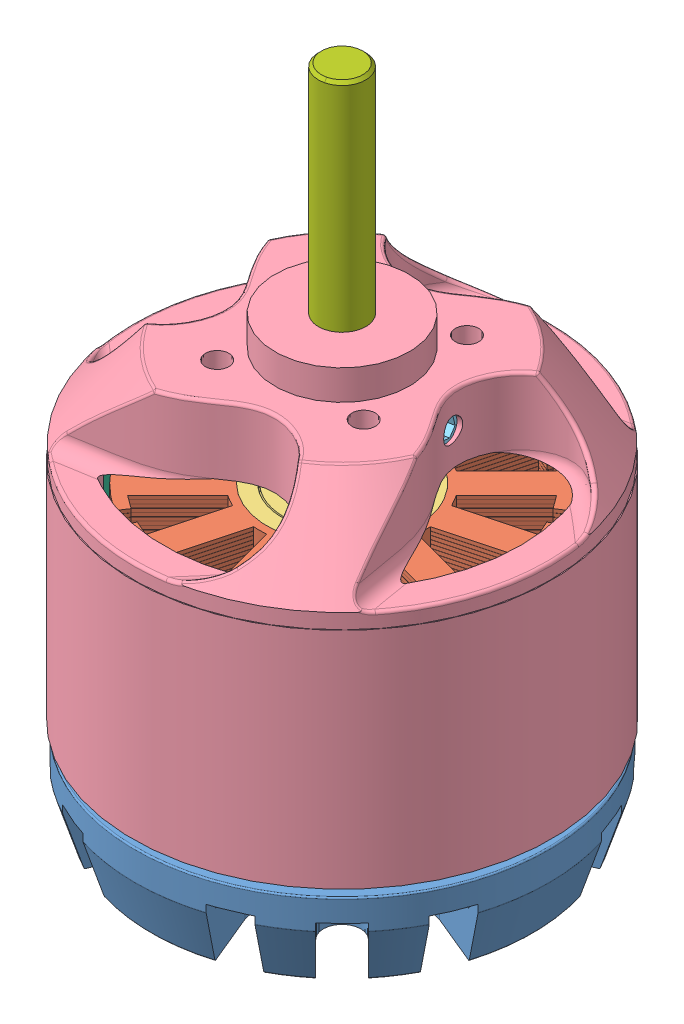
SolidWorks assembly Motore, configuration Default. Lengths in mm.
Overall size (39.3 45 39.3).
60 component instances, 21 part files, 0 mates.
Components (placement in the parent):
- D2830 - Stator-1: D2830 - Stator [Default] at (0 -2 0) x (1 0 0) z (0 1 0) size (39.17 39.17 19.75)
  - Base du stator-1: Base du stator [Default] at (0 0 2) x (0.707107 0.707107 0) z (0 0 1) size (27.7 27.7 8.01)
  - Lamelles du Stator-1: Lamelles du Stator [Default] at (0 0 10) x (0.707107 0.707107 0) z (0 0 1) size (22 22 11.74)
  - Roulement Ó billes-1: Roulement Ó billes [Default] at (0 0 2) x (0.999852 0.017205 0) z (0 0 1) size (10 10 3)
  - Bobine-1: Bobine [Default] at (3.9814 3.9814 9.9) x (0.707107 0.707107 0) z (0 0 1) size (4.61 2.4 12.14) (hidden)
  - Roulement Ó billes-2: Roulement Ó billes [Default] at (0 0 18.74) size (10 10 3)
  - Bobine-2: Bobine [Default] at (1.4573 5.4387 9.9) x (0.258819 0.965926 0) z (0 0 1) size (4.61 2.4 12.14) (hidden)
  - Bobine-3: Bobine [Default] at (-1.4573 5.4387 9.9) x (-0.258819 0.965926 0) z (0 0 1) size (4.61 2.4 12.14) (hidden)
  - Bobine-4: Bobine [Default] at (-3.9814 3.9814 9.9) x (-0.707107 0.707107 0) z (0 0 1) size (4.61 2.4 12.14) (hidden)
  - Bobine-5: Bobine [Default] at (-5.4387 1.4573 9.9) x (-0.965926 0.258819 0) z (0 0 1) size (4.61 2.4 12.14) (hidden)
  - Bobine-6: Bobine [Default] at (-5.4387 -1.4573 9.9) x (-0.965926 -0.258819 0) z (0 0 1) size (4.61 2.4 12.14) (hidden)
  - Bobine-7: Bobine [Default] at (-3.9814 -3.9814 9.9) x (-0.707107 -0.707107 0) z (0 0 1) size (4.61 2.4 12.14) (hidden)
  - Bobine-8: Bobine [Default] at (-1.4573 -5.4387 9.9) x (-0.258819 -0.965926 0) z (0 0 1) size (4.61 2.4 12.14) (hidden)
  - Bobine-9: Bobine [Default] at (1.4573 -5.4387 9.9) x (0.258819 -0.965926 0) z (0 0 1) size (4.61 2.4 12.14) (hidden)
  - Bobine-10: Bobine [Default] at (3.9814 -3.9814 9.9) x (0.707107 -0.707107 0) z (0 0 1) size (4.61 2.4 12.14) (hidden)
  - Bobine-11: Bobine [Default] at (5.4387 -1.4573 9.9) x (0.965926 -0.258819 0) z (0 0 1) size (4.61 2.4 12.14) (hidden)
  - Bobine-12: Bobine [Default] at (5.4387 1.4573 9.9) x (0.965926 0.258819 0) z (0 0 1) size (4.61 2.4 12.14) (hidden)
- D2830 - Rotor-1: D2830 - Rotor [Default] at (-0.1467 -73.15 -0.1528) x (-0.576616 0 0.817016) z (0 1 0) size (28.2 28.2 23.5)
  - Corps supÚrieur-1: Corps supÚrieur [Default] at (0.0403 0.208 79.2501) size (28.2 28.2 23.5)
  - Goupille_M2-1: Goupille_M2 [Default] at (-4.2817 4.4914 98.5001) x (0.495514 0.49998 -0.710272) z (0.710272 -0.703927 0) size (1.7 1.7 4.5)
  - Plaque magnÚtique-1: Plaque magnÚtique [Default] at (5.2017 10.9258 80.2501) x (0.900969 -0.433884 0) z (0 0 1) size (4 1 11.5)
  - Plaque magnÚtique-2: Plaque magnÚtique [Default] at (9.3408 7.6249 80.2501) x (0.62349 -0.781831 0) z (0 0 1) size (4 1 11.5)
  - Plaque magnÚtique-3: Plaque magnÚtique [Default] at (11.6378 2.8551 80.2501) x (0.222521 -0.974928 0) z (0 0 1) size (4 1 11.5)
  - Plaque magnÚtique-4: Plaque magnÚtique [Default] at (11.6378 -2.4391 80.2501) x (-0.222521 -0.974928 0) z (0 0 1) size (4 1 11.5)
  - Plaque magnÚtique-5: Plaque magnÚtique [Default] at (9.3408 -7.2089 80.2501) x (-0.62349 -0.781831 0) z (0 0 1) size (4 1 11.5)
  - Plaque magnÚtique-6: Plaque magnÚtique [Default] at (5.2017 -10.5098 80.2501) x (-0.900969 -0.433884 0) z (0 0 1) size (4 1 11.5)
  - Plaque magnÚtique-7: Plaque magnÚtique [Default] at (0.0403 -11.6878 80.2501) x (-1 0 0) z (0 0 1) size (4 1 11.5)
  - Plaque magnÚtique-8: Plaque magnÚtique [Default] at (-5.1212 -10.5098 80.2501) x (-0.900969 0.433884 0) z (0 0 1) size (4 1 11.5)
  - Plaque magnÚtique-9: Plaque magnÚtique [Default] at (-9.2603 -7.2089 80.2501) x (-0.62349 0.781831 0) z (0 0 1) size (4 1 11.5)
  - Plaque magnÚtique-10: Plaque magnÚtique [Default] at (-11.5573 -2.4391 80.2501) x (-0.222521 0.974928 0) z (0 0 1) size (4 1 11.5)
  - Plaque magnÚtique-11: Plaque magnÚtique [Default] at (-11.5573 2.8551 80.2501) x (0.222521 0.974928 0) z (0 0 1) size (4 1 11.5)
  - Plaque magnÚtique-12: Plaque magnÚtique [Default] at (-9.2603 7.6249 80.2501) x (0.62349 0.781831 0) z (0 0 1) size (4 1 11.5)
  - Plaque magnÚtique-13: Plaque magnÚtique [Default] at (-5.1212 10.9258 80.2501) x (0.900969 0.433884 0) z (0 0 1) size (4 1 11.5)
  - Plaque magnÚtique-14: Plaque magnÚtique [Default] at (0.0403 12.1038 80.2501) size (4 1 11.5)
- Spinner-Part1-1: Spinner-Part1 [Default] at (0 33.1 0) x (0.576616 0 -0.817016) z (0.817016 0 0.576616) size (8.94 36.28 8.94) (hidden)
- Spinner-Part2-1: Spinner-Part2 [Default] at (0 33.1 0) x (0.576616 0 -0.817016) z (0.817016 0 0.576616) size (16 12 16) (hidden)
- Spinner-Part3-1: Spinner-Part3 [Default] at (0 56.1 0) x (0.576616 0 -0.817016) z (0.817016 0 0.576616) size (19.01 24 18.92) (hidden)
- Axe-1: Axe [Default] at (0 -0.9 0) x (0.964595 0 0.263735) z (0 1 0) size (3.17 3.17 45)
- Circlip-1: Circlip [Default] at (0 -0.4 0) x (0.576616 0 -0.817016) z (0 1 0) size (5.59 4.89 0.4)
- FAB_HELICES - 9x4.5 CCW-1: FAB_HELICES - 9x4.5 CCW [Default] at (0 50.6 0) x (-0.817016 0 -0.576616) z (0.576616 0 -0.817016) size (202.02 12.04 179) (hidden)
- CÔble-1: CÔble [Default] at (-4.5922 4.5 -11.0866) x (-0.92388 0 0.382683) z (-0.382683 0 -0.92388) size (2.5 7.25 5.25)
- CÔble-2: CÔble [Default] at (-8.8388 4.5 -8.8388) x (-0.707107 0 0.707107) z (-0.707107 0 -0.707107) size (2.5 7.25 5.25)
- CÔble-3: CÔble [Default] at (-11.0866 4.5 -4.5922) x (-0.382683 0 0.92388) z (-0.92388 0 -0.382683) size (2.5 7.25 5.25)
- CONNECTEUR - Ï3.5 - Moteur-1: CONNECTEUR - Ï3.5 - Moteur [Default] at (-80 0 -8) x (1 0 0) z (0 -1 0) size (13 5 5) (hidden)
- CONNECTEUR - Ï3.5 - Moteur-2: CONNECTEUR - Ï3.5 - Moteur [Default] at (-80 0 0) x (1 0 0) z (0 -1 0) size (13 5 5) (hidden)
- CONNECTEUR - Ï3.5 - Moteur-3: CONNECTEUR - Ï3.5 - Moteur [Default] at (-80 0 8) x (1 0 0) z (0 1 0) size (13 5 5) (hidden)
- PiÞce4^RD - MOTEUR D2830 1100kv-1: PiÞce4^RD - MOTEUR D2830 1100kv [Default] at (-83.5 0 -8) x (0 -1 0) z (-1 0 0) size (5.5 5.5 13) (hidden)
- PiÞce4^RD - MOTEUR D2830 1100kv-2: PiÞce4^RD - MOTEUR D2830 1100kv [Default] at (-83.5 0 8) x (0 -0.964264 0.264942) z (-1 0 0) size (5.5 5.5 13) (hidden)
- PiÞce4^RD - MOTEUR D2830 1100kv-3: PiÞce4^RD - MOTEUR D2830 1100kv [Default] at (-83.5 0 0) x (0 0.521887 -0.853015) z (-1 0 0) size (5.5 5.5 13) (hidden)
- MOTEUR - Support-1: MOTEUR - Support [Default] at (0 -1 0) x (1 0 0) z (0 -1 0) size (40 40 2) (hidden)
- Cable_1-RD - MOTEUR D2830 1000kv-1: Cable_1-RD - MOTEUR D2830 1000kv [Default] at origin size (71.18 4.18 10.39) (hidden)
  - Cble^Cable_1-RD - MOTEUR D2830 1000kv-1: Cble^Cable_1-RD - MOTEUR D2830 1000kv [Default] at origin size (71.18 4.18 10.39)
- Electrical_2-RD - MOTEUR D2830 1000kv-1: Electrical_2-RD - MOTEUR D2830 1000kv [Default] at origin size (74.08 7.31 25.49) (hidden)
  - Cble^Electrical_2-RD - MOTEUR D2830 1000kv-1: Cble^Electrical_2-RD - MOTEUR D2830 1000kv [Default] at origin size (74.08 7.31 25.49)
- Cable_4-RD - MOTEUR D2830 1000kv-1: Cable_4-RD - MOTEUR D2830 1000kv [Default] at origin size (78.89 4.18 16.32) (hidden)
  - Cble^Cable_4-RD - MOTEUR D2830 1000kv-1: Cble^Cable_4-RD - MOTEUR D2830 1000kv [Default] at origin size (78.89 4.18 16.32)
- countersunk flat head cross recess screw_iso_ISO 7046-1 - M2.5 x 6 - Z --- 6C-1: countersunk flat head cross recess screw_iso_ISO 7046-1 - M2.5 x 6 - Z --- 6C [Default] at (-8 -2 0) x (0 1 0) z (0 0 1) size (6 4.7 4.7) (hidden)
- countersunk flat head cross recess screw_iso_ISO 7046-1 - M2.5 x 6 - Z --- 6C-2: countersunk flat head cross recess screw_iso_ISO 7046-1 - M2.5 x 6 - Z --- 6C [Default] at (0 -2 -9.5) x (0 1 0) z (0 0 1) size (6 4.7 4.7) (hidden)
- countersunk flat head cross recess screw_iso_ISO 7046-1 - M2.5 x 6 - Z --- 6C-3: countersunk flat head cross recess screw_iso_ISO 7046-1 - M2.5 x 6 - Z --- 6C [Default] at (8 -2 0) x (0 1 0) z (0 0 1) size (6 4.7 4.7) (hidden)
- countersunk flat head cross recess screw_iso_ISO 7046-1 - M2.5 x 6 - Z --- 6C-4: countersunk flat head cross recess screw_iso_ISO 7046-1 - M2.5 x 6 - Z --- 6C [Default] at (0 -2 9.5) x (0 1 0) z (0 0 1) size (6 4.7 4.7) (hidden)
